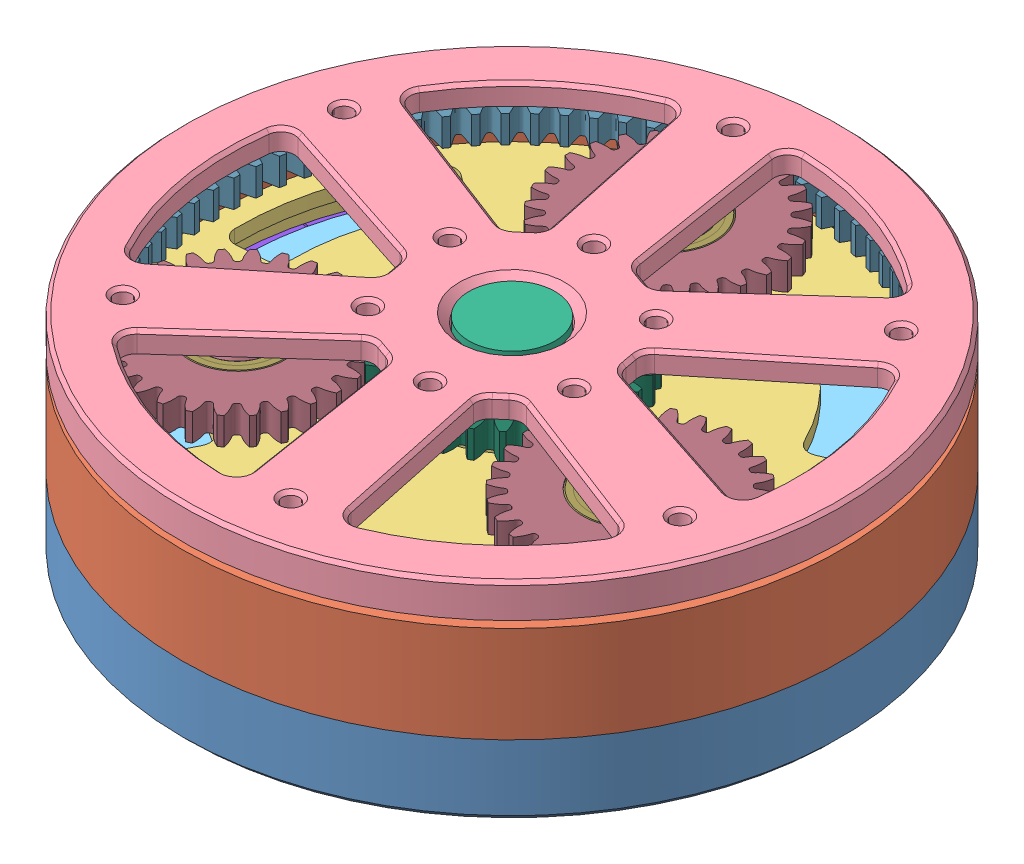
SolidWorks assembly Motor 8, configuration Default. Lengths in mm.
Overall size (136.33 30.6 136.33).
63 component instances, 16 part files, 42 mates.
Components (placement in the parent):
- Housing base-1: Housing base [Default] at origin size (96.7 18.65 96.7)
- Housing cover-1: Housing cover [Default] at origin size (96.7 17.02 96.7)
- Rotor frame-1: Rotor frame [Default] x (-0.232074 0 -0.972698) z (0.972698 0 -0.232074) size (90.2 15.85 90.2)
- Carrier-1: Carrier [Default] x (0.760677 0 -0.649131) z (0.649131 0 0.760677) size (96.7 26.55 96.7)
- Motor core-2: Motor core [Default] at origin size (81 15 81)
- Slipring-1: Slipring [Default] at (0 -1.95 0) x (0.999438 0 0.033536) z (-0.033536 0 0.999438) size (12.6 23.1 12.6)
- PCB-1: PCB [Default] at (0 -10.2 0) size (45 1.2 45)
- Magnet ring-1: Magnet ring [Default] at (0 -6.15 0) x (0.581763 0 -0.813358) z (0.813358 0 0.581763) size (90.2 14.3 90.2)
- Magnetinc position ring-1: Magnetinc position ring [Default] at (0 -6.45 0) x (-0.557963 0 0.829866) z (-0.829866 0 -0.557963) size (13 2.5 13)
- 6803 17x26x5 mm bearing-1: 6803 17x26x5 mm bearing [5972K213] at (0 -1.65 0) x (0.904385 0 -0.426718) z (0 -1 0) size (26 26 5)
- 6803 17x26x5 mm bearing-2: 6803 17x26x5 mm bearing [5972K213] at (0 3.35 0) x (0.954808 0 -0.297225) z (0 -1 0) size (26 26 5)
- 6706 30x37x4 mm bearing-1: 6706 30x37x4 mm bearing [5972K213] at (0 2.15 0) x (0.985684 0 -0.168604) z (0 -1 0) size (37 37 4)
- 6706 30x37x4 mm bearing-2: 6706 30x37x4 mm bearing [5972K213] at (0 6.15 0) x (0.976681 0 0.214697) z (0 -1 0) size (37 37 4)
- 148-2Z-1: 148-2Z [7804K116] at (-21.7546 14 18.5645) x (1 0 0) z (0 -1 0) size (14 14 4)
- 148-2Z-2: 148-2Z [7804K116] at (26.9546 14 9.5578) x (1 0 0) z (0 -1 0) size (14 14 4)
- 148-2Z-3: 148-2Z [7804K116] at (-5.2 14 -28.1223) x (-0.323361 0 0.946276) z (0 -1 0) size (14 14 4)
- Planet Gear M1 Z28 bore 14-3: Planet Gear M1 Z28 bore 14 [GearTrax] at (-21.7546 14 18.5645) x (0.327463 0 0.944864) z (0 1 0) size (30 30 4)
- Planet Gear M1 Z28 bore 14-4: Planet Gear M1 Z28 bore 14 [GearTrax] at (-5.2 14 -28.1223) x (0.992194 0 0.124703) z (0 1 0) size (30 30 4)
- Planet Gear M1 Z28 bore 14-5: Planet Gear M1 Z28 bore 14 [GearTrax] at (26.9546 14 9.5578) x (0.145777 0 0.989317) z (0 1 0) size (30 30 4)
- Ring gear M1 Z85 OD90-1: Ring gear M1 Z85 OD90 [GearTrax] at (0 14 0) x (0.994662 0 0.103189) z (0 -1 0) size (90 90 4)
- Sun Gear M1 Z29 bore 23-1: Sun Gear M1 Z29 bore 23 [GearTrax] at (0 14 0) x (0.991881 0 -0.12717) z (0 -1 0) size (31.2 31.2 4)
- Positioning magnet-1: Positioning magnet [Default] at (-25.7212 7.233 8.2111) size (4 3 4)
- Positioning magnet-2: Positioning magnet [Default] at (-24.2101 7.233 11.9529) x (0.988831 0 -0.149042) z (0.149042 0 0.988831) size (4 3 4)
- Positioning magnet-3: Positioning magnet [Default] at (-22.1582 7.233 15.4277) x (0.955573 0 -0.294755) z (0.294755 0 0.955573) size (4 3 4)
- Positioning magnet-4: Positioning magnet [Default] at (-19.6113 7.233 18.5579) x (0.900969 0 -0.433884) z (0.433884 0 0.900969) size (4 3 4)
- Positioning magnet-5: Positioning magnet [Default] at (-16.6263 7.233 21.2736) x (0.826239 0 -0.56332) z (0.56332 0 0.826239) size (4 3 4)
- Positioning magnet-6: Positioning magnet [Default] at (-13.27 7.233 23.514) x (0.733052 0 -0.680173) z (0.680173 0 0.733052) size (4 3 4)
- Positioning magnet-7: Positioning magnet [Default] at (-9.6172 7.233 25.2291) x (0.62349 0 -0.781831) z (0.781831 0 0.62349) size (4 3 4)
- Positioning magnet-8: Positioning magnet [Default] at (-5.7496 7.233 26.3807) x (0.5 0 -0.866025) z (0.866025 0 0.5) size (4 3 4)
- Positioning magnet-9: Positioning magnet [Default] at (-1.7535 7.233 26.943) x (0.365341 0 -0.930874) z (0.930874 0 0.365341) size (4 3 4)
- Positioning magnet-10: Positioning magnet [Default] at (2.2817 7.233 26.9034) x (0.222521 0 -0.974928) z (0.974928 0 0.222521) size (4 3 4)
- Positioning magnet-11: Positioning magnet [Default] at (6.266 7.233 26.2629) x (0.07473 0 -0.997204) z (0.997204 0 0.07473) size (4 3 4)
- Positioning magnet-12: Positioning magnet [Default] at (10.1103 7.233 25.0356) x (-0.07473 0 -0.997204) z (0.997204 0 -0.07473) size (4 3 4)
- Positioning magnet-13: Positioning magnet [Default] at (13.7287 7.233 23.2491) x (-0.222521 0 -0.974928) z (0.974928 0 -0.222521) size (4 3 4)
- Positioning magnet-14: Positioning magnet [Default] at (17.0405 7.233 20.9433) x (-0.365341 0 -0.930874) z (0.930874 0 -0.365341) size (4 3 4)
- Positioning magnet-15: Positioning magnet [Default] at (19.9716 7.233 18.1696) x (-0.5 0 -0.866025) z (0.866025 0 -0.5) size (4 3 4)
- Positioning magnet-16: Positioning magnet [Default] at (22.4566 7.233 14.9901) x (-0.62349 0 -0.781831) z (0.781831 0 -0.62349) size (4 3 4)
- Positioning magnet-17: Positioning magnet [Default] at (24.4399 7.233 11.4757) x (-0.733052 0 -0.680173) z (0.680173 0 -0.733052) size (4 3 4)
- Positioning magnet-18: Positioning magnet [Default] at (25.8773 7.233 7.7049) x (-0.826239 0 -0.56332) z (0.56332 0 -0.826239) size (4 3 4)
- Positioning magnet-19: Positioning magnet [Default] at (26.7366 7.233 3.762) x (-0.900969 0 -0.433884) z (0.433884 0 -0.900969) size (4 3 4)
- Positioning magnet-20: Positioning magnet [Default] at (26.9987 7.233 -0.2649) x (-0.955573 0 -0.294755) z (0.294755 0 -0.955573) size (4 3 4)
- Positioning magnet-21: Positioning magnet [Default] at (26.6577 7.233 -4.2858) x (-0.988831 0 -0.149042) z (0.149042 0 -0.988831) size (4 3 4)
- Positioning magnet-22: Positioning magnet [Default] at (25.7212 7.233 -8.2111) x (-1 0 0) z (0 0 -1) size (4 3 4)
- Positioning magnet-23: Positioning magnet [Default] at (24.2101 7.233 -11.9529) x (-0.988831 0 0.149042) z (-0.149042 0 -0.988831) size (4 3 4)
- Positioning magnet-24: Positioning magnet [Default] at (22.1582 7.233 -15.4277) x (-0.955573 0 0.294755) z (-0.294755 0 -0.955573) size (4 3 4)
- Positioning magnet-25: Positioning magnet [Default] at (19.6113 7.233 -18.5579) x (-0.900969 0 0.433884) z (-0.433884 0 -0.900969) size (4 3 4)
- Positioning magnet-26: Positioning magnet [Default] at (16.6263 7.233 -21.2736) x (-0.826239 0 0.56332) z (-0.56332 0 -0.826239) size (4 3 4)
- Positioning magnet-27: Positioning magnet [Default] at (13.27 7.233 -23.514) x (-0.733052 0 0.680173) z (-0.680173 0 -0.733052) size (4 3 4)
- Positioning magnet-28: Positioning magnet [Default] at (9.6172 7.233 -25.2291) x (-0.62349 0 0.781831) z (-0.781831 0 -0.62349) size (4 3 4)
- Positioning magnet-29: Positioning magnet [Default] at (5.7496 7.233 -26.3807) x (-0.5 0 0.866025) z (-0.866025 0 -0.5) size (4 3 4)
- Positioning magnet-30: Positioning magnet [Default] at (1.7535 7.233 -26.943) x (-0.365341 0 0.930874) z (-0.930874 0 -0.365341) size (4 3 4)
- Positioning magnet-31: Positioning magnet [Default] at (-2.2817 7.233 -26.9034) x (-0.222521 0 0.974928) z (-0.974928 0 -0.222521) size (4 3 4)
- Positioning magnet-32: Positioning magnet [Default] at (-6.266 7.233 -26.2629) x (-0.07473 0 0.997204) z (-0.997204 0 -0.07473) size (4 3 4)
- Positioning magnet-33: Positioning magnet [Default] at (-10.1103 7.233 -25.0356) x (0.07473 0 0.997204) z (-0.997204 0 0.07473) size (4 3 4)
- Positioning magnet-34: Positioning magnet [Default] at (-13.7287 7.233 -23.2491) x (0.222521 0 0.974928) z (-0.974928 0 0.222521) size (4 3 4)
- Positioning magnet-35: Positioning magnet [Default] at (-17.0405 7.233 -20.9433) x (0.365341 0 0.930874) z (-0.930874 0 0.365341) size (4 3 4)
- Positioning magnet-36: Positioning magnet [Default] at (-19.9716 7.233 -18.1696) x (0.5 0 0.866025) z (-0.866025 0 0.5) size (4 3 4)
- Positioning magnet-37: Positioning magnet [Default] at (-22.4566 7.233 -14.9901) x (0.62349 0 0.781831) z (-0.781831 0 0.62349) size (4 3 4)
- Positioning magnet-38: Positioning magnet [Default] at (-24.4399 7.233 -11.4757) x (0.733052 0 0.680173) z (-0.680173 0 0.733052) size (4 3 4)
- Positioning magnet-39: Positioning magnet [Default] at (-25.8773 7.233 -7.7049) x (0.826239 0 0.56332) z (-0.56332 0 0.826239) size (4 3 4)
- Positioning magnet-40: Positioning magnet [Default] at (-26.7366 7.233 -3.762) x (0.900969 0 0.433884) z (-0.433884 0 0.900969) size (4 3 4)
- Positioning magnet-41: Positioning magnet [Default] at (-26.9987 7.233 0.2649) x (0.955573 0 0.294755) z (-0.294755 0 0.955573) size (4 3 4)
- Positioning magnet-42: Positioning magnet [Default] at (-26.6577 7.233 4.2858) x (0.988831 0 0.149042) z (-0.149042 0 0.988831) size (4 3 4)
Mates (geometry in assembly coordinates):
- Coincident1: coincident: line of Motor core-2 through (69.0457 0 0) axis (0 0 1); line of Slipring-1 through (69.0457 0 -1.95) axis (0 0 1)
- Concentric1: concentric: cylinder of PCB-1 through (0 -9 0) axis (0 -1 0) radius 3.5; line of assembly
- Parallel1: parallel: plane of PCB-1 through (0 -10.2 0) normal (0 0 1); plane of assembly through (0 0 0) normal (0 0 1)
- Coincident2: coincident: line of Magnet ring-1 through (69.0457 0 -6.15) axis (0 0 1); line of assembly
- Width1: width: plane of Magnet ring-1 through (-3.3765 6.15 40.66) normal (0 1 0); plane of Magnet ring-1 through (5.4432 -6.15 40.4353) normal (0 -1 0); plane of Motor core-2 through (-40.5 6 0) normal (0 1 0); plane of Motor core-2 through (-40.5 -6 0) normal (0 -1 0)
- Coincident3: coincident: line of Magnetinc position ring-1 through (69.0457 0 -6.45) axis (0 0 1); line of assembly
- Distance3: distance = 3 mm: plane of Motor core-2 through (-40.5 -6 0) normal (0 -1 0); plane of PCB-1 through (-11.5 -9 11.5) normal (0 1 0)
- Coincident4: coincident: plane of Rotor frame-1 through (0 0 0) normal (0 1 0); plane of assembly through (0 0 0) normal (0 1 0)
- Coincident5: coincident: line of Rotor frame-1 through (0 0 0) axis (0 1 0); line of assembly
- Coincident6: coincident: plane of Carrier-1 through (0 0 0) normal (0 1 0); plane of assembly through (0 0 0) normal (0 1 0)
- Coincident7: coincident: line of Carrier-1 through (0 0 0) axis (0 1 0); line of assembly
- Concentric2: concentric: cylinder of 6803 17x26x5 mm bearing-1 through (0 -4.15 0) axis (0 -1 0) radius 8.5; line of Carrier-1 through (0 0 0) axis (0 1 0)
- Concentric3: concentric: cylinder of 6803 17x26x5 mm bearing-2 through (0 0.85 0) axis (0 -1 0) radius 8.5; line of Carrier-1 through (0 0 0) axis (0 1 0)
- Coincident15: coincident: line of 6803 17x26x5 mm bearing-1 through (0 0.85 0) axis (0 1 0); line of assembly
- Concentric4: concentric: cylinder of 6706 30x37x4 mm bearing-1 through (0 0.15 0) axis (0 -1 0) radius 15; line of assembly
- Concentric5: concentric: cylinder of 6706 30x37x4 mm bearing-2 through (0 4.15 0) axis (0 -1 0) radius 15; line of assembly
- Coincident28: coincident: plane of Carrier-1 through (-5.0205 -3.95 4.2843) normal (0 -1 0); plane of Magnetinc position ring-1 through (3.6268 -3.95 -5.3941) normal (0 1 0)
- Coincident298: coincident: plane of ?; plane of assembly through (0 0 0) normal (0 0 1)
- Concentric32: concentric: cylinder of 148-2Z-1 through (-21.7546 12 18.5645) axis (0 -1 0) radius 4; cylinder of Carrier-1 through (-21.7546 12.1363 18.5645) axis (0 1 0) radius 5.2
- Coincident321: coincident: plane of Carrier-1 through (-25.7101 16 21.94) normal (0 -1 0); plane of 148-2Z-1 through (-21.7546 16 22.7645) normal (0 1 0)
- Concentric33: concentric: cylinder of Planet Gear M1 Z28 bore 14-4 through (-5.2 14 -28.1223) axis (0 1 0) radius 7; cylinder of 148-2Z-3 through (-5.2 12 -28.1223) axis (0 -1 0) radius 4
- Coincident322: coincident: plane of Carrier-1 through (31.8556 16 11.2956) normal (0 -1 0); plane of 148-2Z-2 through (26.9546 16 13.7578) normal (0 1 0)
- Concentric34: concentric: cylinder of 148-2Z-2 through (26.9546 12 9.5578) axis (0 -1 0) radius 4; line of Planet Gear M1 Z28 bore 14-5 through (26.9546 69 9.5578) axis (0 -1 0)
- Concentric35: concentric: cylinder of 148-2Z-2 through (26.9546 12 9.5578) axis (0 -1 0) radius 4; cylinder of Carrier-1 through (26.9546 12.1363 9.5578) axis (0 1 0) radius 5.2
- Concentric36: concentric: cylinder of 148-2Z-1 through (-21.7546 12 18.5645) axis (0 -1 0) radius 4; cylinder of Carrier-1 through (-21.7546 12.1363 18.5645) axis (0 1 0) radius 5.2
- Concentric37: concentric: cylinder of 148-2Z-1 through (-21.7546 12 18.5645) axis (0 -1 0) radius 4; cylinder of Planet Gear M1 Z28 bore 14-3 through (-21.7546 14 18.5645) axis (0 1 0) radius 7
- Coincident327: coincident: plane of Carrier-1 through (-6.1455 16 -33.2356) normal (0 -1 0); plane of 148-2Z-3 through (-9.1744 16 -29.4804) normal (0 1 0)
- Concentric44: concentric: cylinder of 148-2Z-3 through (-5.2 12 -28.1223) axis (0 -1 0) radius 4; cylinder of Carrier-1 through (-5.2 12.1363 -28.1223) axis (0 1 0) radius 5.2
- Coincident328: coincident: plane of Carrier-1 through (-4.9444 -1.95 4.2194) normal (0 1 0); plane of Slipring-1 through (-2.4986 -1.95 -0.0838) normal (0 -1 0)
- Coincident329: coincident: plane of 6803 17x26x5 mm bearing-1 through (3.7338 0.85 7.9134) normal (0 1 0); plane of 6803 17x26x5 mm bearing-2 through (3.0414 0.85 9.7702) normal (0 -1 0)
- Coincident330: coincident: plane of Housing base-1 through (-5.4339 5.85 0) normal (0 1 0); plane of 6803 17x26x5 mm bearing-2 through (3.7896 5.85 12.1738) normal (0 1 0)
- Coincident332: coincident: plane of 6706 30x37x4 mm bearing-1 through (2.5712 4.15 15.0317) normal (0 1 0); plane of 6706 30x37x4 mm bearing-2 through (-3.5067 4.15 15.9523) normal (0 -1 0)
- Coincident333: coincident: plane of Housing base-1 through (-13 8.15 0) normal (0 1 0); plane of 6706 30x37x4 mm bearing-2 through (-3.2741 8.15 14.8944) normal (0 1 0)
- Distance4: distance = 1 mm: plane of Housing base-1 through (-29.23 6.233 0) normal (0 1 0); plane of Positioning magnet-1 through (-25.7212 7.233 8.2111) normal (0 -1 0)
- Concentric45: concentric: cylinder of Rotor frame-1 through (-25.7212 0.15 8.2111) axis (0 1 0) radius 2.06; cylinder of Positioning magnet-1 through (-25.7212 10.233 8.2111) axis (0 -1 0) radius 2
- Coincident334: coincident: line of Ring gear M1 Z85 OD90-1 through (0 -41 0) axis (0 1 0); line of assembly
- Coincident335: coincident: plane of Rotor frame-1 through (2.6688 16 11.186) normal (0 1 0); plane of Ring gear M1 Z85 OD90-1 through (-4.6435 16 44.7598) normal (0 1 0)
- Coincident336: coincident: line of Sun Gear M1 Z29 bore 23-1 through (0 -41 0) axis (0 1 0); line of assembly
- Coincident337: coincident: plane of Rotor frame-1 through (2.6688 16 11.186) normal (0 1 0); plane of Sun Gear M1 Z29 bore 23-1 through (1.9838 16 15.4733) normal (0 1 0)
- Coincident338: coincident: plane of Planet Gear M1 Z28 bore 14-5 through (26.9546 16 9.5578) normal (0 1 0); plane of Sun Gear M1 Z29 bore 23-1 through (1.9838 16 15.4733) normal (0 1 0)
- Coincident339: coincident: plane of Planet Gear M1 Z28 bore 14-3 through (-21.7546 16 18.5645) normal (0 1 0); plane of Sun Gear M1 Z29 bore 23-1 through (1.9838 16 15.4733) normal (0 1 0)
- Coincident340: coincident: plane of Planet Gear M1 Z28 bore 14-4 through (-5.2 16 -28.1223) normal (0 1 0); plane of Sun Gear M1 Z29 bore 23-1 through (1.9838 16 15.4733) normal (0 1 0)
